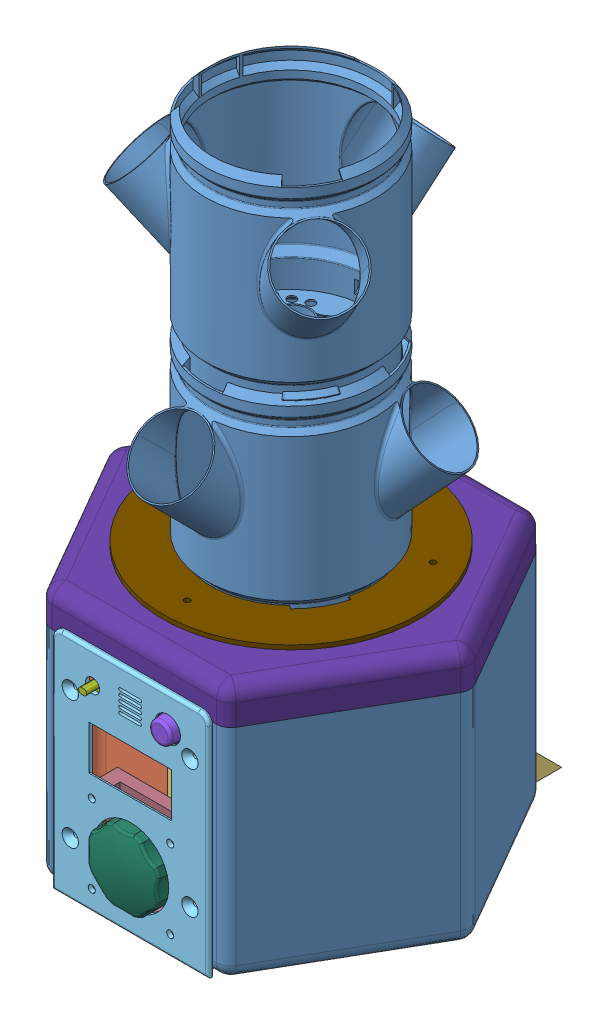
SolidWorks assembly Assy_final, configuration Predeterminado. Lengths in mm.
Overall size (251.55 471.54 285.79).
26 component instances, 19 part files, 7 mates.
Components (placement in the parent):
- Assy_base_tanque-1: Assy_base_tanque [Default] at (-175.8753 -85.0418 -202.911) size (250.94 210.12 285.79)
  - base  1_1-1: base  1_1 [Default] at (121.3241 94.324 202.911) size (250.94 155 220)
  - Assy_box_control-1: Assy_box_control [Default] at (251.8598 45.2792 -150.6249) size (110 187.12 285.79)
    - box-control_D-1: box-control_D [Default] at (-180.6357 49.0448 463.5359) size (50.1 155 250)
    - box-control_I-1: box-control_I [Default] at (-82.0357 49.0448 463.5359) size (50.1 155 250)
    - base_control_box-1: base_control_box [Default] at (-178.5357 49.0448 465.1037) size (96 25 220)
    - frente_control_box-1: frente_control_box [Default] at (-185.5357 49.0448 463.5359) size (110 160 8.5)
    - DS3231 RTC-2: DS3231 RTC [Default] at (-98.9357 55.5448 310.9359) x (0 0 -1) z (0 -1 0) size (44.75 22.8 13.53)
      - Default-1: Default [Predeterminado] at origin size (44.75 22.8 13.53)
    - LDR-1: LDR [Default] at (-156.876 173.9735 458.6019) x (1 0 0) z (0 0 -1) size (14.2 40.8 21.6)
    - MQ135_sensor-1: MQ135_sensor [Default] at (-98.6357 185.4448 458.0359) x (0 1 0) z (0 0 1) size (36.7 20 20.1)
    - ESP32_breadboard-1: ESP32_breadboard [Predeterminado] at (-142.2857 27.4234 204.8986) x (0 0 -1) z (1 0 0) size (186.74 40.42 55.48)
      - placa breadboard-1: placa breadboard [Predeterminado] at (-172.7373 28.1214 24.25) size (136 1.8 48.5)
      - 20-Pin Header - Female - 2.54mm-1: 20-Pin Header - Female - 2.54mm [Predeterminado] at (-93.0773 29.9214 11.43) size (51.3 8 2.5)
      - 20-Pin Header - Female - 2.54mm-2: 20-Pin Header - Female - 2.54mm [Predeterminado] at (-93.0773 29.9214 -11.43) size (51.3 8 2.5)
      - PCB_ESP32-38Pines-1: PCB_ESP32-38Pines [Predeterminado] at (-67.3173 36.9214 0) x (0 0 -1) z (1 0 0) size (28 10.12 55.48)
    - perilla-1: perilla [Predeterminado] at (-127.2204 86.8536 424.0509) size (65 65 36.44)
      - Rotary Encoder - KY-040-1: Rotary Encoder - KY-040 [Default] at (-4.2339 1.2762 17.985) size (19 30.75 32.39)
      - chasis_perilla-1: chasis_perilla [Predeterminado] at (-2.6839 3.7912 27.485) size (65 65 20.5)
      - rodamiento-1: rodamiento [Predeterminado] at (-2.6839 3.7912 33.485) x (1 0 0) z (0 -1 0) size (44.2 9 44.2)
      - perilla52-1: perilla52 [Predeterminado] at (-2.6839 3.7912 47.635) x (1 0 0) z (0 0 -1) size (52.46 52.46 20)
    - LoRa_Module_RA-02-1: LoRa_Module_RA-02 [Predeterminado] at (-94.5357 55.5448 278.6359) x (1 0 0) z (0 1 0) size (16 17 3.03)
  - techo_tanque-1: techo_tanque [Predeterminado] at (121.3241 274.324 202.911) x (1 0 0) z (0 0 -1) size (250.94 30 220)
  - embudo-1: embudo [Predeterminado] at (121.3241 277.324 202.911) x (0 -1 0) z (-0.5 0 0.866025) size (41.28 180 180)
- cup_holder_fer-1: cup_holder_fer [Default] at (-54.5513 7398.8094 0) x (0.903374 0 -0.428853) z (0 -1 0) size (160.92 177.88 148)
- cup_holder_fer-2: cup_holder_fer [Default] at (-54.5513 7531.8094 0) x (0.08029 0 -0.996772) z (0 -1 0) size (160.92 177.88 148)
Mates (geometry in assembly coordinates):
- Concéntrica1: concentric anti-aligned: cylinder of Assy_base_tanque-1/embudo-1 through (-54.5513 238.316 0) axis (0 1 0) radius 56.0128; cylinder of cup_holder_fer-1 through (-54.5513 -414.2776 0) axis (0 -1 0) radius 55
- Concéntrica2: concentric aligned: cylinder of cup_holder_fer-1 through (-54.5513 -414.2776 0) axis (0 -1 0) radius 55; cylinder of cup_holder_fer-2 through (-54.5513 -281.2776 0) axis (0 -1 0) radius 55
- Coincidente1: coincident anti-aligned: plane of Assy_base_tanque-1/embudo-1 through (-54.5513 192.2822 0) normal (0.64805 0 0.761597); plane of cup_holder_fer-1 through (-54.5513 7398.8094 0) normal (-0.64805 0 -0.761597)
- Coincidente2: coincident anti-aligned: plane of Assy_base_tanque-1/embudo-1 through (-6.0538 192.2822 28) normal (0 1 0); circle of cup_holder_fer-1
- Coincidente3: coincident anti-aligned: plane of cup_holder_fer-1 through (-54.5513 7398.8094 0) normal (-0.335538 0 0.942027); plane of cup_holder_fer-2 through (-54.5513 7531.8094 0) normal (0.335538 0 -0.942027)
- Distancia1: distance = 132 mm anti-aligned: plane of cup_holder_fer-2 through (-54.5513 305.6964 0) normal (0 -1 0); plane of cup_holder_fer-1 through (-54.5513 173.6964 0) normal (0 1 0)
- Simétrico1: symmetric aligned: plane of Assy_base_tanque-1/techo_tanque-1 through (8.9573 164.2822 110) normal (0 0 1); plane of Assy_base_tanque-1/techo_tanque-1 through (-118.0598 164.2822 -110) normal (0 0 -1)
